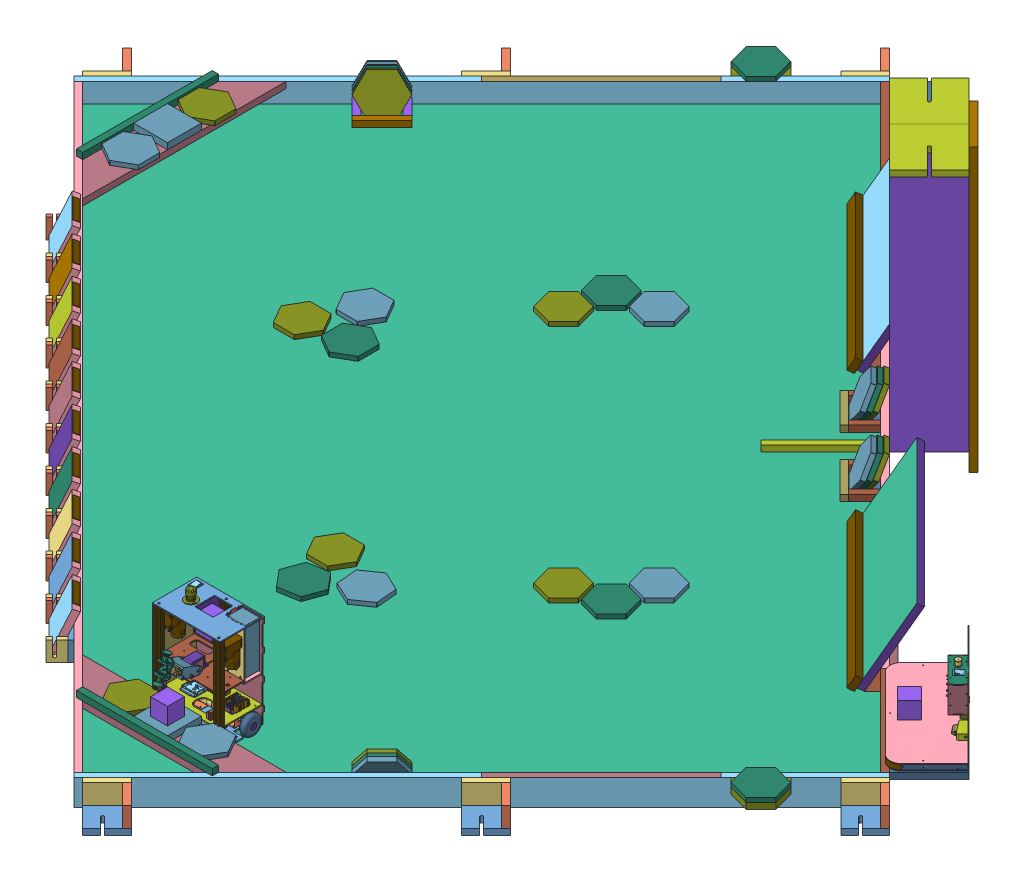
SolidWorks assembly Farid, configuration Default. Lengths in mm. (continued)
Components (placement in the parent): (continued)
- réplique-1: réplique [Default] at (173.8286 323.1947 656.2469) size (60 60 60)
- IBT-2 (module only)-1: IBT-2 (module only) [Default] at (112.5786 356.2835 564.3969) x (-1 0 0) z (0 0 1) size (51 40.62 49.7)
- IBT-2 (module only)-2: IBT-2 (module only) [Default] at (235.0786 361.6831 564.3969) size (51 40.62 49.7)
- support etage-1: support etage [Default] at (173.8286 274.8594 487.2468) x (1 0 0) z (0 1 0) size (19 14 15)
- support etage-2: support etage [Default] at (279.8286 272.9465 600.2469) x (-1 0 0) z (0 1 0) size (19 14 15)
- support etage-3: support etage [Default] at (67.8286 274.8594 600.2469) x (-1 0 0) z (0 1 0) size (19 14 15)
- réplique-3: réplique [Default] at (173.8286 500.6326 497.2468) size (60 60 60)
- support replique-1: support replique [Default] at (173.8286 466.6326 512.7469) x (-1 0 0) z (0 1 0) size (75 91 4)
- support etage-4: support etage [Default] at (173.8286 466.6326 487.2468) x (1 0 0) z (0 1 0) size (19 14 15)
- support etage-5: support etage [Default] at (163.8286 466.6326 477.2468) x (0 0 1) z (0 1 0) size (19 14 15)
- support etage-6: support etage [Default] at (183.8286 466.6326 477.2468) x (0 0 -1) z (0 1 0) size (19 14 15)
- support etage-7: support etage [Default] at (67.8286 379.2835 600.2469) x (-1 0 0) z (0 1 0) size (19 14 15)
- support etage-8: support etage [Default] at (279.8286 379.2835 600.2469) x (-1 0 0) z (0 1 0) size (19 14 15)
- support etage-9: support etage [Default] at (173.8286 379.2835 487.2468) x (1 0 0) z (0 1 0) size (19 14 15)
- etage lateral-1: etage lateral [Default] at (54.0286 394.8594 545.2469) x (0 0 -1) z (1 0 0) size (157 330 4)
- etage lateral-2: etage lateral [Default] at (289.6286 394.8594 545.2469) x (0 0 -1) z (1 0 0) size (157 330 4) (hidden)
- couvert arriere-1: couvert arriere [Default] at (184.7377 364.8594 463.2469) size (240 330 4)
- lipo battery-1: lipo battery [Default] at (255.0286 544.8594 497.2469) x (0 0 -1) z (0 -1 0) size (52 61 162)
- ventouse_final-1: ventouse_final [Default] at (157.6946 390.9623 703.4797) x (-0.185088 -0.33986 -0.922083) z (0.982722 -0.06401 -0.173667) size (30 42.25 32)
- ventouse_final-2: ventouse_final [Default] at (157.6946 474.5584 672.668) x (-0.167275 0.340962 0.925075) z (0.98591 0.05785 0.156953) size (30 42.25 32)
- e-stop 61-3440.stp-1: e-stop 61-3440.stp [Default] at (114.0286 534.8094 543.2469) x (-0.937891 0 -0.346929) z (0 1 0) size (43 43 76.4)
- couvert lateral replique-1: couvert lateral replique [Default] at (210.3286 505.7476 512.7469) x (0 0 1) z (-1 0 0) size (91 78.23 4)
- couvert lateral replique-2: couvert lateral replique [Default] at (141.3286 505.7476 512.7469) x (0 0 1) z (-1 0 0) size (91 78.23 4)
- profilé-1: profilé [Default] at (67.8286 364.8594 610.2469) x (1 0 0) z (0 -1 0) size (20 20 330)
- profilé-2: profilé [Default] at (279.8286 364.8594 610.2469) x (1 0 0) z (0 -1 0) size (20 20 330)
- profilé-3: profilé [Default] at (173.8286 364.8594 477.2469) x (1 0 0) z (0 -1 0) size (20 20 330)
- PompeVide-AirpoD2028B-12vdc-4: PompeVide-AirpoD2028B-12vdc [Défaut] at (77.3286 514.8594 552.1469) x (1 0 0) z (0 -1 0) size (38.6 62.4 92)
- roof-1: roof [Default] at (174.0286 548.8594 541.7469) x (1 0 0) z (0 -1 0) size (240 157 4)
- couvert lateral batterie-1: couvert lateral batterie [Default] at (216.0286 459.8594 497.2469) x (0 0 -1) z (1 0 0) size (63.8 174 4)
- couvert lateral batterie_2-1: couvert lateral batterie_2 [Default] at (255.0286 459.8594 531.2469) x (-1 0 0) z (0 0 -1) size (73.8 174 4)
- floor battery-1: floor battery [Default] at (252.5286 370.8594 497.0469) x (1 0 0) z (0 1 0) size (75.4 70 4)
- interrupteur principal-1: interrupteur principal [Défaut] at (76.5286 548.8594 489.2469) x (0 0 1) z (-1 0 0) size (32 33.35 25)
- support_ventouse-1: support_ventouse [Default] at (157.6946 417.7476 693.6072) x (1 0 0) z (0 -0.938295 0.345835) size (35 26 4)
- support_ventouse-2: support_ventouse [Default] at (157.6946 451.5263 681.1571) x (1 0 0) z (0 -0.938295 0.345835) size (35 26 4)
- Assemblage1-1: Assemblage1 [Défaut] at (1585.9209 359.1947 -743.419) x (0.707107 0 0.707107) z (-0.707107 0 0.707107) size (440 246.17 210.2)
  - Pièce1-1: Pièce1 [Défaut] at origin size (440 156 3)
  - Pièce2-1: Pièce2 [Défaut] at (0 -85 105) x (-1 0 0) z (0 -1 0) size (439 210 3)
  - Part10 - Copie-1: Part10 - Copie [Default] at (-51.8676 -60.5031 49.9498) size (122.5 87.5 7.03)
  - Pièce9-1: Pièce9 [Défaut] at (-219.5 -76.5 104.5) x (0 0 -1) z (1 0 0) size (167 17 3)
  - Pièce6-2: Pièce6 [Défaut] at (-80 -76.5 207) size (359 17 3)
  - réplique-1: réplique [Default] at (0 -35 119.6611) size (60 60 60)
  - Pièce9-3: Pièce9 [Défaut] at (216.5 -76.5 104.5) x (0 0 -1) z (1 0 0) size (167 17 3)
  - Long Range SHARP IR Sensors - #GP2Y0A21YK0F-1: Long Range SHARP IR Sensors - #GP2Y0A21YK0F [Default] at (14.75 -35.3157 15.7) x (-1 0 0) z (0 0 1) size (44.5 18.9 13.5)
  - moraba3 3ordh-1: moraba3 3ordh [Défaut] at (-64.25 21.25 28) x (0 -1 0) z (1 0 0) size (93.5 53 3)
  - moraba3 3ordh-2: moraba3 3ordh [Défaut] at (61.25 21.25 27.8) x (0 -1 0) z (1 0 0) size (93.5 53 3)
  - moraba3 toul-2: moraba3 toul [Défaut] at (0 -25.5 28) x (1 0 0) z (0 1 0) size (128.5 53 3)
  - moraba3 toul loutaa-1: moraba3 toul loutaa [Défaut] at (0 65 28) x (1 0 0) z (0 1 0) size (128.5 53 3)
  - impr3d-1: impr3d [Défaut] at (0 -65 18) x (1 0 0) z (0 1 0) size (52 19 39.5)
  - FixAngle-1: FixAngle [Défaut] at (-216.5 -85 3) size (30 8 30)
  - FixAngle-2: FixAngle [Défaut] at (-61.25 -22.5 3) x (0 1 0) z (1 0 0) size (30 8 30)
  - FixAngle-3: FixAngle [Défaut] at (61.25 -22.5 3) x (-1 0 0) z (0 1 0) size (30 8 30)
  - FixAngle-4: FixAngle [Défaut] at (-61.25 65 3) x (1 0 0) z (0 -1 0) size (30 8 30)
  - FixAngle-5: FixAngle [Défaut] at (61.25 65 3) x (0 -1 0) z (-1 0 0) size (30 8 30)
  - FixAngle-9: FixAngle [Défaut] at (-61.25 -22.5 50.9) x (1 0 0) z (0 1 0) size (30 8 30)
  - FixAngle-10: FixAngle [Défaut] at (-61.25 65 50.9) x (0 -1 0) z (1 0 0) size (30 8 30)
  - FixAngle-11: FixAngle [Défaut] at (61.25 65 50.9) x (-1 0 0) z (0 -1 0) size (30 8 30)
  - FixAngle-12: FixAngle [Défaut] at (61.25 -22.5 50.9) x (0 1 0) z (-1 0 0) size (30 8 30)
  - arc_vitrine-1: arc_vitrine [Default] at (-219.5 -68 170) x (1 0 0) z (0 -1 0) size (50 50 17)
  - arc_vitrine-3: arc_vitrine [Default] at (179.5 -68 210) x (0 0 -1) z (0 -1 0) size (50 50 17)
  - support etage-1: support etage [Default] at (-216.5 -68 115) x (0 0 -1) z (0 1 0) size (19 14 15)
  - interrupteur principal-1: interrupteur principal [Défaut] at (13.25 68 26.5) x (0 0 -1) z (1 0 0) size (32 33.35 25)
  - FixAngle-13: FixAngle [Défaut] at (216.5 -85 3) x (0 0 1) z (-1 0 0) size (30 8 30)
  - support etage-3: support etage [Default] at (-77 -85 3) x (-1 0 0) z (0 -1 0) size (19 14 15)
  - support etage-4: support etage [Default] at (77 -85 3) x (-1 0 0) z (0 -1 0) size (19 14 15)
  - support etage-5: support etage [Default] at (216.5 -68 115) x (0 0 1) z (0 1 0) size (19 14 15)
  - Arduino UNO-1: Arduino UNO [Predeterminado] at (-140.4953 -85 41.7907) x (0 0 1) z (-1 0 0) size (74.8 15.1 53.3)
  - 5V One Channel Relay.step-1: 5V One Channel Relay.step [Default] at (-146.5 -85 84.8) x (0 0 1) z (-1 0 0) size (25.5 18.75 51)
  - support etage-6: support etage [Default] at (-22 -45.25 3) x (0 1 0) z (-1 0 0) size (19 14 15)
  - support etage-7: support etage [Default] at (22 -45.25 3) x (0 -1 0) z (1 0 0) size (19 14 15)
  - Force stop button-1: Force stop button [По умолчанию] at (-19.9998 66.9329 27.9999) x (0.906121 0 -0.423019) z (0 -1 0) size (20.79 20.79 48.92)
  - floor-1: floor [Default] at (0 -65 106.5) x (1 0 0) z (0 -1 0) size (439 207 3)
  - support etage-8: support etage [Default] at (0 -68 207) x (-1 0 0) z (0 1 0) size (19 14 15)
  - systeme de fixation-1: systeme de fixation [Défaut] at (0 -135 104.7444) x (-0.92707 0 -0.374889) z (-0.374889 0 0.92707) size (50.29 25 49.34)
  - fixation tige-1: fixation tige [Défaut] at (0 -85 104.7444) x (0.5 0 -0.866025) z (0.866025 0 0.5) size (13 55.5 15.01)
  - Long Range SHARP IR Sensors - #GP2Y0A21YK0F-2: Long Range SHARP IR Sensors - #GP2Y0A21YK0F [Default] at (122.0333 -35.3157 24.7506) x (-0.992278 0 -0.124035) z (-0.124035 0 0.992278) size (44.5 18.9 13.5)
  - support sharp lateral-1: support sharp lateral [Default] at (107.2359 -41.8157 3) size (60 20 29.34)
  - support sharp lateral-2: support sharp lateral [Default] at (-107.2359 -41.8157 3) x (-1 0 0) z (0 0 1) size (60 20 29.34)
  - Long Range SHARP IR Sensors - #GP2Y0A21YK0F-3: Long Range SHARP IR Sensors - #GP2Y0A21YK0F [Default] at (-92.7611 -35.3157 21.0916) x (-0.992278 0 0.124035) z (0.124035 0 0.992278) size (44.5 18.9 13.5)
- system wheel-1: system wheel [Default] at (266.7722 228.3737 520.7342) x (0 -0.852789 -0.522255) z (1 0 0) size (69.5 69.5 30.5)
  - part1-1: part1 [Default] at (0.5601 15.4113 33.6689) size (21.5 21.5 11)
  - part2-1: part2 [Default] at (0.5601 15.4113 5.1689) x (0 1 0) z (0 0 -1) size (21.5 21.5 18)
  - _gomme-1: _gomme [Default] at (0.5601 15.4113 11.6689) size (69.5 69.5 22)
- support_switch-1: support_switch [Default] at (77.8286 298.3527 609.7469) x (0 0 1) z (0 -1 0) size (29 9 24.5)
- support_switch-2: support_switch [Default] at (269.8286 322.8527 609.7469) x (0 0 1) z (0 1 0) size (29 9 24.5)
- system wheel-2: system wheel [Default] at (80.8851 227.4184 520.1492) x (0 0.852789 0.522255) z (-1 0 0) size (69.5 69.5 30.5)
  - part1-1: part1 [Default] at (0.5601 15.4113 33.6689) size (21.5 21.5 11)
  - part2-1: part2 [Default] at (0.5601 15.4113 5.1689) x (0 1 0) z (0 0 -1) size (21.5 21.5 18)
  - _gomme-1: _gomme [Default] at (0.5601 15.4113 11.6689) size (69.5 69.5 22)
- BillePorteuse-1: BillePorteuse [Défaut] at (173.8286 208.7594 609.7469) x (-0.837169 0 -0.546944) z (-0.546944 0 0.837169) size (31 21 31)
- capteur fin de course-1: capteur fin de course [Default] at (83.8286 310.6027 626.6239) x (0 -1 0) z (1 0 0) size (20 14 6)
- capteur fin de course-2: capteur fin de course [Default] at (257.8286 310.6027 626.6239) x (0 -1 0) z (1 0 0) size (20 14 6)
Mates (geometry in assembly coordinates):
- Coincident33: coincident anti-aligned: plane of étage 3-1 through (169.8286 383.2835 544.2469) normal (0 1 0); plane of Servo-1 through (150.2867 383.2835 566.2469) normal (0 -1 0)
- Concentric1: concentric anti-aligned: cylinder of Servo-1 through (146.7867 399.2835 597.2469) axis (1 0 0) radius 9.5; cylinder of bras_replique-1 through (146.7867 399.2835 597.2469) axis (-1 0 0) radius 12.5
- Coincident66: coincident anti-aligned: plane of Servo-1 through (146.7867 399.2835 597.2469) normal (-1 0 0); plane of bras_replique-1 through (146.7867 399.2835 597.2469) normal (1 0 0)
- Width3: width anti-aligned: plane of Servo Motor MG996R _米字摇臂.step-3 through (187.7367 422.9819 635.086) normal (1 0 0); plane of Servo Motor MG996R _米字摇臂.step-3 through (147.8367 405.8111 641.4148) normal (-1 0 0); plane of bras_replique-1 through (188.7867 399.2835 597.2469) normal (-1 0 0); plane of bras_replique-1 through (146.7867 399.2835 597.2469) normal (1 0 0)
- Width5: width anti-aligned: plane of support servo kbyr-1 through (151.5367 383.2835 566.2469) normal (0 0 1); plane of Servo-1 through (151.5367 405.2835 609.2469) normal (0 0 -1); plane of support servo kbyr-1 through (150.2867 383.2835 566.2469) normal (0 0 -1); plane of Servo-1 through (150.2867 383.2835 609.2469) normal (0 0 1)
- Width6: width aligned: plane of support servo kbyr-1 through (181.5367 409.2835 603.2469) normal (1 0 0); plane of Servo-1 through (151.5367 409.2835 603.2469) normal (-1 0 0); plane of support servo kbyr-1 through (182.7867 399.2835 587.7469) normal (1 0 0); plane of Servo-1 through (150.2867 399.2835 587.7469) normal (-1 0 0)
- Coincident75: coincident anti-aligned: plane of Servo-1 through (150.2867 415.2835 566.2469) normal (0 1 0); plane of support servo kbyr-1 through (151.5367 415.2835 566.2469) normal (0 -1 0)
- Distance3: distance = 3 mm anti-aligned: plane of étage 3-1 through (289.8286 383.2835 629.2469) normal (0 0 1); plane of TABLE_2021.step-1/Distributeurs.step-1/DistributeurCoin_1.step-1/Taquet.step-1 through (534.4531 249.1947 626.2469) normal (0 0 -1)
- Width7: width anti-aligned: plane of étage 3-1 through (289.8286 383.2835 467.2469) normal (1 0 0); plane of TABLE_2021.step-1/Distributeurs.step-1/DistributeurCoin_1.step-1/SupportStatuette.step-1 through (57.8286 383.2835 467.2469) normal (-1 0 0); plane of étage 3-1 through (113.8286 271.1947 626.2469) normal (-1 0 0); plane of TABLE_2021.step-1/Distributeurs.step-1/DistributeurCoin_1.step-1/SupportStatuette.step-1 through (233.8286 271.1947 746.2469) normal (1 0 0)
- Coincident81: coincident anti-aligned: plane of TABLE_2021.step-1/Distributeurs.step-1/DistributeurCoin_1.step-1/SupportStatuette.step-1 through (173.8286 293.1947 686.2469) normal (0 1 0); plane of réplique-1 through (143.8286 293.1947 716.2469) normal (0 -1 0)
- Width8: width anti-aligned: plane of réplique-1 through (203.8286 353.1947 716.2469) normal (1 0 0); plane of TABLE_2021.step-1/Distributeurs.step-1/DistributeurCoin_1.step-1/SupportStatuette.step-1 through (143.8286 353.1947 716.2469) normal (-1 0 0); plane of réplique-1 through (113.8286 271.1947 626.2469) normal (-1 0 0); plane of TABLE_2021.step-1/Distributeurs.step-1/DistributeurCoin_1.step-1/SupportStatuette.step-1 through (233.8286 271.1947 746.2469) normal (1 0 0)
- Width9: width aligned: plane of réplique-1 through (173.8286 323.1947 656.2469) normal (0 0 -1); plane of TABLE_2021.step-1/Distributeurs.step-1/DistributeurCoin_1.step-1/Taquet.step-1 through (173.8286 323.1947 716.2469) normal (0 0 1); plane of réplique-1 through (534.4531 249.1947 626.2469) normal (0 0 -1); plane of TABLE_2021.step-1/Distributeurs.step-1/DistributeurCoin_1.step-1/Taquet (1).step-1 through (414.4531 271.1947 746.2469) normal (0 0 -1)
- Parallel1: parallel aligned: plane of étage 3-1 through (169.8286 379.2835 544.2469) normal (0 -1 0); plane of IBT-2 (module only)-1 through (112.5786 354.6835 564.3969) normal (0 -1 0)
- Coincident87: coincident anti-aligned: plane of étage 3-1 through (169.8286 379.2835 544.2469) normal (0 -1 0); plane of IBT-2 (module only)-1 through (107.5231 379.2835 582.5719) normal (0 1 0)
- Parallel2: parallel aligned: plane of étage 3-1 through (57.8286 383.2835 467.2469) normal (-1 0 0); plane of IBT-2 (module only)-1 through (87.0786 356.2835 582.5719) normal (-1 0 0)
- Distance6: distance = 30 mm aligned: plane of étage 3-1 through (57.8286 383.2835 467.2469) normal (-1 0 0); plane of IBT-2 (module only)-1 through (87.8286 354.6835 586.7569) normal (-1 0 0)
- Coincident91: coincident anti-aligned: plane of robot_sghyr-1/etage electronique-1 through (173.8286 274.8594 547.2469) normal (0 -1 0); plane of support etage-1 through (183.3286 274.8594 487.2468) normal (0 1 0)
- Coincident94: coincident anti-aligned: plane of robot_sghyr-1/etage electronique-1 through (173.8286 274.8594 547.2469) normal (0 -1 0); plane of support etage-3 through (58.3286 274.8594 600.2469) normal (0 1 0)
- Coincident97: coincident anti-aligned: plane of support replique-1 through (173.8286 466.6326 512.7469) normal (0 -1 0); plane of support etage-4 through (183.3286 466.6326 487.2468) normal (0 1 0)
- Coincident101: coincident anti-aligned: plane of support replique-1 through (173.8286 466.6326 512.7469) normal (0 -1 0); plane of support etage-6 through (183.8286 466.6326 467.7468) normal (0 1 0)
- Width19: width anti-aligned: plane of réplique-3 through (203.8286 530.6326 557.2468) normal (1 0 0); plane of support replique-1 through (143.8286 530.6326 557.2468) normal (-1 0 0); plane of réplique-3 through (141.3286 470.6326 558.2469) normal (-1 0 0); plane of support replique-1 through (206.3286 470.6326 558.2469) normal (1 0 0)
- Coincident102: coincident anti-aligned: plane of réplique-3 through (143.8286 470.6326 557.2468) normal (0 -1 0); plane of support replique-1 through (173.8286 470.6326 512.7469) normal (0 1 0)
- Coincident104: coincident anti-aligned: plane of étage 3-1 through (169.8286 379.2835 544.2469) normal (0 -1 0); plane of support etage-7 through (58.3286 379.2835 600.2469) normal (0 1 0)
- Coincident106: coincident anti-aligned: plane of étage 3-1 through (169.8286 379.2835 544.2469) normal (0 -1 0); plane of support etage-8 through (270.3286 379.2835 600.2469) normal (0 1 0)
- Coincident108: coincident anti-aligned: plane of étage 3-1 through (169.8286 379.2835 544.2469) normal (0 -1 0); plane of support etage-9 through (183.3286 379.2835 487.2468) normal (0 1 0)
- Coincident112: coincident anti-aligned: plane of robot_sghyr-1/base_robot_sghyr-1 through (173.8286 214.8594 547.2469) normal (0 1 0); plane of etage lateral-1 through (58.0286 214.8594 620.2469) normal (0 -1 0)
- Coincident115: coincident anti-aligned: plane of robot_sghyr-1/base_robot_sghyr-1 through (173.8286 214.8594 547.2469) normal (0 1 0); plane of couvert arriere-1 through (53.8286 214.8594 467.2469) normal (0 -1 0)
- Coincident116: coincident aligned: plane of robot_sghyr-1/base_robot_sghyr-1 through (53.8286 214.8594 462.2469) normal (-1 0 0); plane of couvert arriere-1 through (53.8286 544.8594 467.2469) normal (-1 0 0)
- Coincident125: coincident aligned: plane of couvert lateral replique-1 through (206.3286 466.6326 467.2469) normal (0 -1 0); plane of support replique-1 through (173.8286 466.6326 512.7469) normal (0 -1 0)
- Coincident127: coincident anti-aligned: plane of couvert arriere-1 through (184.7377 364.8594 467.2469) normal (0 0 1); plane of couvert lateral replique-1 through (206.3286 544.8626 467.2469) normal (0 0 -1)
- Coincident130: coincident anti-aligned: plane of support replique-1 through (206.3286 470.6326 558.2469) normal (1 0 0); plane of couvert lateral replique-1 through (206.3286 505.7476 512.7469) normal (-1 0 0)
- Concentric9: concentric anti-aligned: cylinder of robot_sghyr-1/base_robot_sghyr-1 through (67.8286 214.8594 610.2469) axis (0 -1 0) radius 2.5; cylinder of profilé-1 through (67.8286 214.8594 610.2469) axis (0 1 0) radius 2.5
- Coincident131: coincident anti-aligned: plane of robot_sghyr-1/base_robot_sghyr-1 through (173.8286 214.8594 547.2469) normal (0 1 0); plane of profilé-1 through (66.3248 214.8594 616.3469) normal (0 -1 0)
- Concentric10: concentric anti-aligned: cylinder of robot_sghyr-1/base_robot_sghyr-1 through (173.8286 214.8594 477.2469) axis (0 -1 0) radius 2.5; cylinder of profilé-3 through (173.8286 214.8594 477.2469) axis (0 1 0) radius 2.5
- Coincident132: coincident anti-aligned: plane of robot_sghyr-1/base_robot_sghyr-1 through (173.8286 214.8594 547.2469) normal (0 1 0); plane of profilé-3 through (172.3248 214.8594 483.3469) normal (0 -1 0)
- Coincident133: coincident aligned: plane of etage lateral-2 through (293.6286 544.8594 620.2469) normal (0 0 1); plane of profilé-2 through (289.4286 214.8594 620.2469) normal (0 0 1)
- Coincident137: coincident anti-aligned: plane of etage lateral-2 through (289.6286 394.8594 545.2469) normal (-1 0 0); plane of couvert arriere-1 through (289.6286 255.0594 467.2469) normal (1 0 0)
- Coincident138: coincident aligned: plane of etage lateral-2 through (293.6286 544.8594 463.2469) normal (0 0 -1); plane of couvert arriere-1 through (184.7377 364.8594 463.2469) normal (0 0 -1)
- Coincident139: coincident anti-aligned: plane of robot_sghyr-1/etage electronique-1 through (289.8286 274.8594 467.2469) normal (0 0 -1); plane of couvert arriere-1 through (184.7377 364.8594 467.2469) normal (0 0 1)
- Coincident148: coincident anti-aligned: plane of PompeVide-AirpoD2028B-12vdc-1 through (289.6286 475.8594 595.2469) normal (1 0 0); plane of etage lateral-2 through (289.6286 394.8594 545.2469) normal (-1 0 0)
- Distance11: distance = 30 mm aligned: plane of PompeVide-AirpoD2028B-12vdc-1 through (289.6286 514.8594 532.8469) normal (0 1 0); plane of etage lateral-2 through (293.6286 544.8594 620.2469) normal (0 1 0)
- Distance12: distance = 5 mm anti-aligned: plane of PompeVide-AirpoD2028B-12vdc-1 through (251.0286 475.8594 595.2469) normal (0 0 1); plane of profilé-2 through (270.2286 214.8594 600.2469) normal (0 0 -1)
- Coincident154: coincident anti-aligned: plane of profilé-1 through (66.3248 544.8594 616.3469) normal (0 1 0); plane of roof-1 through (174.0286 544.8594 541.7469) normal (0 -1 0)
- Coincident155: coincident aligned: plane of etage lateral-1 through (54.0286 394.8594 545.2469) normal (-1 0 0); plane of roof-1 through (54.0286 544.8594 620.2469) normal (-1 0 0)
- Coincident156: coincident aligned: plane of profilé-1 through (77.4286 214.8594 620.2469) normal (0 0 1); plane of roof-1 through (54.0286 544.8594 620.2469) normal (0 0 1)
- Width27: width anti-aligned: plane of roof-1 through (216.0286 544.8594 487.2469) normal (0 0 1); plane of couvert lateral batterie-1 through (220.0286 544.8594 507.2469) normal (0 0 -1); plane of roof-1 through (220.0286 548.8594 487.3469) normal (0 0 -1); plane of couvert lateral batterie-1 through (220.0286 544.8594 507.1469) normal (0 0 1)
- Coincident157: coincident anti-aligned: plane of roof-1 through (216.0286 544.8594 507.2469) normal (1 0 0); plane of couvert lateral batterie-1 through (216.0286 459.8594 497.2469) normal (-1 0 0)
- Coincident158: coincident aligned: plane of roof-1 through (174.0286 548.8594 541.7469) normal (0 1 0); plane of couvert lateral batterie-1 through (220.0286 548.8594 507.1469) normal (0 1 0)
- Width28: width anti-aligned: plane of couvert lateral batterie_2-1 through (264.9286 544.8594 527.2469) normal (1 0 0); plane of roof-1 through (245.1286 548.8594 527.2469) normal (-1 0 0); plane of couvert lateral batterie_2-1 through (245.0286 544.8594 531.2469) normal (1 0 0); plane of roof-1 through (265.0286 544.8594 527.2469) normal (-1 0 0)
- Coincident159: coincident aligned: plane of roof-1 through (174.0286 548.8594 541.7469) normal (0 1 0); plane of couvert lateral batterie_2-1 through (264.9286 548.8594 527.2469) normal (0 1 0)
- Coincident160: coincident anti-aligned: plane of roof-1 through (265.0286 544.8594 531.2469) normal (0 0 -1); plane of couvert lateral batterie_2-1 through (255.0286 459.8594 531.2469) normal (0 0 1)
- Width29: width aligned: plane of lipo battery-1 through (224.5286 382.8594 523.2469) normal (-1 0 0); plane of roof-1 through (285.5286 382.8594 523.2469) normal (1 0 0); plane of lipo battery-1 through (290.0286 544.8594 467.2469) normal (-1 0 0); plane of roof-1 through (220.0286 544.8594 507.2469) normal (1 0 0)
- Width30: width aligned: plane of roof-1 through (220.0286 544.8594 467.2469) normal (0 0 1); plane of lipo battery-1 through (220.0286 544.8594 527.2469) normal (0 0 -1); plane of roof-1 through (285.5286 382.8594 523.2469) normal (0 0 1); plane of lipo battery-1 through (285.5286 382.8594 471.2469) normal (0 0 -1)
- Concentric11: concentric aligned: cylinder of e-stop 61-3440.stp-1 through (114.0286 552.9094 543.2469) axis (0 1 0) radius 12; cylinder of roof-1 through (114.0286 544.8594 543.2469) axis (0 1 0) radius 7.5
- Coincident161: coincident anti-aligned: plane of e-stop 61-3440.stp-1 through (114.0286 548.8594 543.2469) normal (0 -1 0); plane of roof-1 through (174.0286 548.8594 541.7469) normal (0 1 0)
- Distance13: distance = 4 mm aligned: plane of lipo battery-1 through (255.0286 544.8594 497.2469) normal (0 1 0); plane of roof-1 through (174.0286 548.8594 541.7469) normal (0 1 0)
- Distance14: distance = 40 mm aligned: plane of IBT-2 (module only)-2 through (212.8286 363.2831 589.2469) normal (0 0 1); plane of étage 3-1 through (289.8286 383.2835 629.2469) normal (0 0 1)
- Coincident163: coincident anti-aligned: plane of couvert lateral batterie_2-1 through (289.9286 374.8594 527.2469) normal (0 -1 0); plane of floor battery-1 through (252.5286 374.8594 497.0469) normal (0 1 0)
- Coincident164: coincident aligned: plane of couvert lateral batterie-1 through (216.0286 459.8594 497.2469) normal (-1 0 0); plane of floor battery-1 through (216.0286 374.8594 467.2469) normal (-1 0 0)
- Coincident165: coincident anti-aligned: plane of couvert arriere-1 through (184.7377 364.8594 467.2469) normal (0 0 1); plane of floor battery-1 through (216.0286 374.8594 467.2469) normal (0 0 -1)
- Coincident166: coincident anti-aligned: plane of roof-1 through (174.0286 548.8594 541.7469) normal (0 1 0); plane of interrupteur principal-1 through (76.5286 548.8594 489.2469) normal (0 -1 0)
- Parallel4: parallel anti-aligned: plane of roof-1 through (54.0286 544.8594 620.2469) normal (-1 0 0); plane of interrupteur principal-1 through (89.0286 550.8594 473.2469) normal (1 0 0)
- Distance15: distance = 10 mm aligned: plane of interrupteur principal-1 through (64.0286 550.8594 473.2469) normal (0 0 -1); plane of roof-1 through (54.0286 544.8594 463.2469) normal (0 0 -1)
- Distance16: distance = 10 mm aligned: plane of interrupteur principal-1 through (64.0286 550.8594 473.2469) normal (-1 0 0); plane of roof-1 through (54.0286 544.8594 620.2469) normal (-1 0 0)
- Coincident173: coincident anti-aligned: plane of support_ventouse-1 through (162.6946 410.1903 684.6693) normal (0 -0.345835 -0.938295); plane of SUPPORT VENTOUSE-1 through (147.0974 405.4988 686.3985) normal (0 0.345835 0.938295)
- Concentric12: concentric anti-aligned: cylinder of ventouse_final-1 through (157.6946 390.9623 703.4797) axis (0 -0.938295 0.345835) radius 6.5; cylinder of support_ventouse-1 through (157.6946 413.9945 694.9905) axis (0 0.938295 -0.345835) radius 6.5
- Coincident174: coincident anti-aligned: plane of ventouse_final-1 through (157.6946 413.9945 694.9905) normal (0 0.938295 -0.345835); plane of support_ventouse-1 through (157.6946 413.9945 694.9905) normal (0 -0.938295 0.345835)
- Coincident175: coincident anti-aligned: plane of SUPPORT VENTOUSE-1 through (157.6946 426.1895 670.2462) normal (-1 0 0); plane of support_ventouse-1 through (157.6946 417.7476 693.6072) normal (1 0 0)
- Width31: width anti-aligned: plane of SUPPORT VENTOUSE-1 through (144.6839 398.0406 680.6213) normal (0 -0.938295 0.345835); plane of bras_replique-1 through (144.6839 454.3384 659.8712) normal (0 0.938295 -0.345835); plane of SUPPORT VENTOUSE-1 through (146.7867 414.2963 591.7135) normal (0 0.938295 -0.345835); plane of bras_replique-1 through (146.7867 384.2708 602.7802) normal (0 -0.938295 0.345835)
- Concentric13: concentric aligned: cylinder of ventouse_final-2 through (157.6946 474.5584 672.668) axis (0 0.938295 -0.345835) radius 6.5; cylinder of support_ventouse-2 through (157.6946 447.7731 682.5405) axis (0 0.938295 -0.345835) radius 6.5
- Distance18: distance = 10 mm aligned: plane of support_ventouse-1 through (157.6946 413.9945 694.9905) normal (0 -0.938295 0.345835); plane of SUPPORT VENTOUSE-1 through (144.6839 398.0406 680.6213) normal (0 -0.938295 0.345835)
- Coincident181: coincident anti-aligned: plane of ventouse_final-2 through (157.6946 451.5263 681.1571) normal (0 -0.938295 0.345835); plane of support_ventouse-2 through (157.6946 451.5263 681.1571) normal (0 0.938295 -0.345835)
- Coincident182: coincident anti-aligned: plane of TABLE_2021.step-1/BaseTable.step-1/ExperimentZone.step-2 through (1515.2102 271.1947 -672.7083) normal (0 1 0); plane of Assemblage1-1/Pièce2-1 through (1511.6747 271.1947 -669.1728) normal (0 -1 0)
- Coincident184: coincident aligned: plane of TABLE_2021.step-1/BaseTable.step-1/ExperimentZone.step-2 through (1589.4564 271.1947 -739.8834) normal (0.707107 0 -0.707107); plane of Assemblage1-1/Pièce1-1 through (1585.9209 359.1947 -743.419) normal (0.707107 0 -0.707107)
- Coincident187: coincident anti-aligned: plane of SUPPORT VENTOUSE-1 through (157.6946 426.1895 670.2462) normal (-1 0 0); plane of Access_HS-645_BrasRondPetitModele-1 through (157.6946 428.4796 668.8693) normal (1 0 0)
- Coincident188: coincident anti-aligned: plane of SUPPORT VENTOUSE-1 through (135.2376 455.7217 663.6244) normal (0 -0.345835 -0.938295); plane of Access_HS-645_BrasRondPetitModele-1 through (161.4446 430.0359 673.0916) normal (0 0.345835 0.938295)
- Concentric15: concentric aligned: cylinder of robot_sghyr-1/pololu-37D-encoder-1 through (273.1411 235.8594 507.2469) axis (-1 0 0) radius 3; cylinder of system wheel-1/accoupelement court-1 through (272.1411 235.8594 507.2469) axis (-1 0 0) radius 3
- Coincident189: coincident anti-aligned: plane of profilé-1 through (77.8286 214.8594 619.8469) normal (1 0 0); plane of support_switch-1 through (77.8286 322.8527 619.2469) normal (-1 0 0)
- Coincident192: coincident aligned: plane of profilé-1 through (77.4286 214.8594 600.2469) normal (0 0 -1); plane of support_switch-1 through (77.8286 298.3527 600.2469) normal (0 0 -1)
- Distance21: distance = 2 mm anti-aligned: plane of system wheel-1/accoupelement court-2 through (260.1411 235.9447 507.2991) normal (-1 0 0); plane of robot_sghyr-1/pololu-37D-encoder-1 through (258.1411 235.8594 507.2469) normal (1 0 0)
- Tangent1: tangent: circle of TABLE_2021.step-1/BaseTable.step-1/Ground.step-1; circle of system wheel-2/_gomme-1
- Concentric16: concentric aligned: cylinder of étage 3-1 through (174.5367 379.2835 621.2469) axis (0 1 0) radius 2.5; cylinder of support servo kbyr-1 through (174.5367 383.2835 621.2469) axis (0 1 0) radius 2
- Parallel6: parallel anti-aligned: plane of robot_sghyr-1/base_robot_sghyr-1 through (173.8286 209.8594 547.2469) normal (0 -1 0); plane of TABLE_2021.step-1/BaseTable.step-1/Ground.step-1 through (-179.7247 201.1947 -780.8956) normal (0 1 0)
- Concentric17: concentric aligned: cylinder of robot_sghyr-1/Robot2015_support bille porteuse-1 through (173.8286 226.8594 609.7469) axis (0 -1 0) radius 11.9; cylinder of BillePorteuse-1 through (173.8286 201.2594 609.7469) axis (0 -1 0) radius 12
- Coincident193: coincident anti-aligned: plane of robot_sghyr-1/Robot2015_support bille porteuse-1 through (173.8286 210.7594 609.7469) normal (0 -1 0); plane of BillePorteuse-1 through (183.8747 210.7594 616.3102) normal (0 1 0)
- Coincident194: coincident anti-aligned: plane of support_switch-1 through (83.8286 322.8527 619.2469) normal (1 0 0); plane of capteur fin de course-1 through (83.8286 310.6027 626.6239) normal (-1 0 0)
- Width36: width anti-aligned: plane of capteur fin de course-1 through (89.8286 320.6027 621.6239) normal (0 1 0); plane of support_switch-1 through (89.8286 300.6027 621.6239) normal (0 -1 0); plane of capteur fin de course-1 through (86.8286 320.8527 600.2469) normal (0 -1 0); plane of support_switch-1 through (86.8286 300.3527 600.2469) normal (0 1 0)
- Width37: width anti-aligned: plane of Servo Motor MG996R _米字摇臂.step-3 through (187.0367 405.1543 641.6568) normal (0 -0.938295 0.345835); plane of bras_replique-1 through (148.5367 423.6387 634.8439) normal (0 0.938295 -0.345835); plane of Servo Motor MG996R _米字摇臂.step-3 through (96.3387 400.3748 632.0148) normal (0 0.938295 -0.345835); plane of bras_replique-1 through (96.3387 432.0841 654.4319) normal (0 -0.938295 0.345835)
- Coincident195: coincident anti-aligned: plane of Servo Motor MG996R _米字摇臂.step-3 through (194.5472 415.6404 660.4926) normal (0 -0.345835 -0.938295); plane of bras_replique-1 through (146.7867 421.7628 658.2361) normal (0 0.345835 0.938295)
- Tangent2: tangent aligned: cylinder of Access_HS-645_BrasRondPetitModele-1 through (157.6946 428.4796 668.8693) axis (0 -0.345835 -0.938295) radius 2.75; cylinder of Servo Motor MG996R _米字摇臂.step-3 through (157.6867 426.0166 669.7771) axis (0 -0.345835 -0.938295) radius 5.375
- Coincident196: coincident anti-aligned: plane of Servo Motor MG996R _米字摇臂.step-3 through (157.6867 426.0166 669.7771) normal (0 0.345835 0.938295); plane of Access_HS-645_BrasRondPetitModele-1 through (162.1946 428.4796 668.8693) normal (0 -0.345835 -0.938295)
- Concentric19: concentric anti-aligned: cylinder of étage 3-1 through (158.5367 379.2835 621.2469) axis (0 1 0) radius 2.5; cylinder of support servo kbyr-1 through (158.5367 396.2835 621.2469) axis (0 -1 0) radius 3
